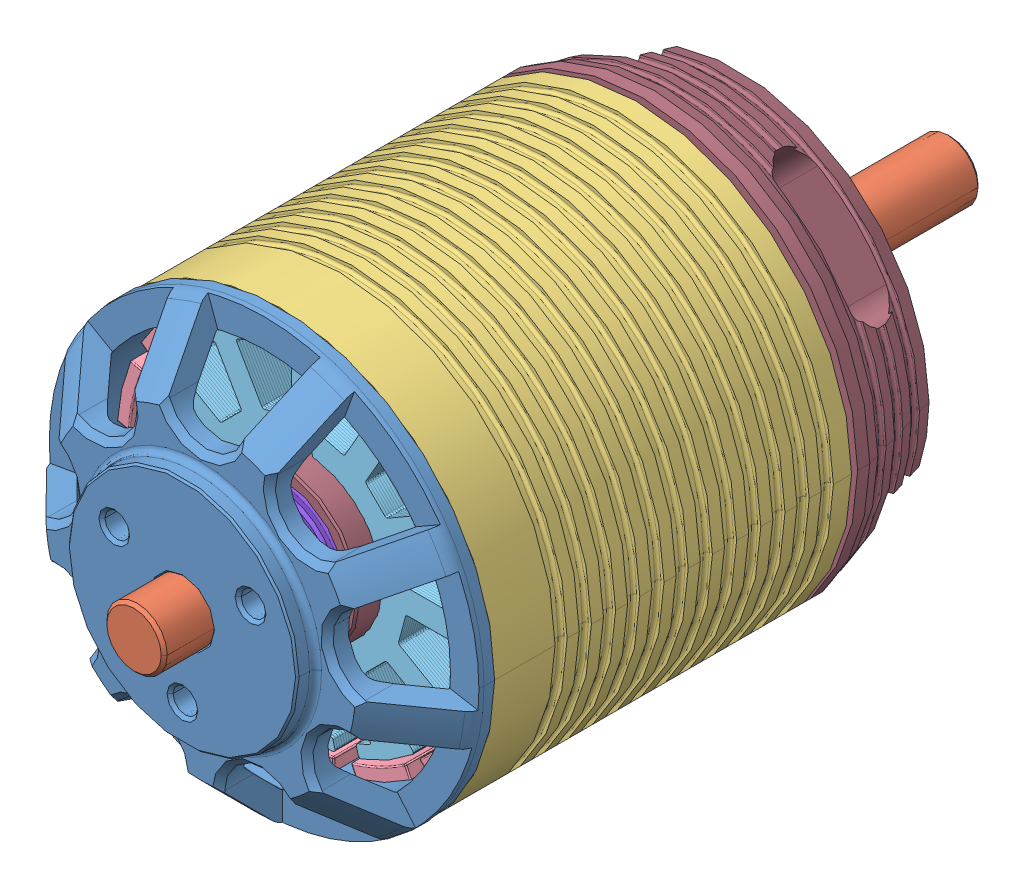
SolidWorks assembly BA-2826-Motor, configuration Default. Lengths in mm. (continued)
Components (placement in the parent): (continued)
- BA-2826-Motor(2)^BA-2826-Motor-1: BA-2826-Motor(2)^BA-2826-Motor [Default] at origin size (35.6 35.6 67.5) (virtual) (continued)
  - 2826-Stator-Mount^BA-2826-Motor(2)_BA-2826-Motor-1: 2826-Stator-Mount^BA-2826-Motor(2)_BA-2826-Motor [Default] at (-12.4646 -13.2477 18.5701) size (35.6 35.6 38.01) (virtual) (continued)
    - 28x13x26mm-Stator^2826-Stator-Mount_BA-2826-Motor(2)_BA-2826-Motor-1: 28x13x26mm-Stator^2826-Stator-Mount_BA-2826-Motor(2)_BA-2826-Motor [Default] at (-35.5349 -3.2376 -36.4185) size (28 28 26) (virtual) (continued)
      - 28x13x5mm-Stator^28x13x26mm-Stator_2826-Stator-Mount_BA-2826-Motor(2)_BA-2826-Motor-4: 28x13x5mm-Stator^28x13x26mm-Stator_2826-Stator-Mount_BA-2826-Motor(2)_BA-2826-Motor [Default] at (6.5198 12.3714 10.0893) size (28 28 5) (virtual)
        - 28x13x1mm-Stator^28x13x5mm-Stator_28x13x26mm-Stator_2826-Stator-Mount_BA-2826-Motor(2)_BA-2826-Motor-1: 28x13x1mm-Stator^28x13x5mm-Stator_28x13x26mm-Stator_2826-Stator-Mount_BA-2826-Motor(2)_BA-2826-Motor [Default] at (34.0086 1.4103 18.4307) size (28 28 1) (virtual)
          - 28x13-Stator Plate^28x13x1mm-Stator_28x13x5mm-Stator_28x13x26mm-Stator_2826-Stator-Mount_BA-2826-Motor(2)_BA-2826-Motor-1: 28x13-Stator Plate^28x13x1mm-Stator_28x13x5mm-Stator_28x13x26mm-Stator_2826-Stator-Mount_BA-2826-Motor(2)_BA-2826-Motor [Default] at (-28.2175 12.5042 6.2948) size (28 28 0.2) (virtual)
          - 28x13-Stator Plate^28x13x1mm-Stator_28x13x5mm-Stator_28x13x26mm-Stator_2826-Stator-Mount_BA-2826-Motor(2)_BA-2826-Motor-2: 28x13-Stator Plate^28x13x1mm-Stator_28x13x5mm-Stator_28x13x26mm-Stator_2826-Stator-Mount_BA-2826-Motor(2)_BA-2826-Motor [Default] at (-28.2175 12.5042 6.0948) size (28 28 0.2) (virtual)
          - 28x13-Stator Plate^28x13x1mm-Stator_28x13x5mm-Stator_28x13x26mm-Stator_2826-Stator-Mount_BA-2826-Motor(2)_BA-2826-Motor-3: 28x13-Stator Plate^28x13x1mm-Stator_28x13x5mm-Stator_28x13x26mm-Stator_2826-Stator-Mount_BA-2826-Motor(2)_BA-2826-Motor [Default] at (-28.2175 12.5042 5.8948) size (28 28 0.2) (virtual)
          - 28x13-Stator Plate^28x13x1mm-Stator_28x13x5mm-Stator_28x13x26mm-Stator_2826-Stator-Mount_BA-2826-Motor(2)_BA-2826-Motor-4: 28x13-Stator Plate^28x13x1mm-Stator_28x13x5mm-Stator_28x13x26mm-Stator_2826-Stator-Mount_BA-2826-Motor(2)_BA-2826-Motor [Default] at (-28.2175 12.5042 5.6948) size (28 28 0.2) (virtual)
          - 28x13-Stator Plate^28x13x1mm-Stator_28x13x5mm-Stator_28x13x26mm-Stator_2826-Stator-Mount_BA-2826-Motor(2)_BA-2826-Motor-5: 28x13-Stator Plate^28x13x1mm-Stator_28x13x5mm-Stator_28x13x26mm-Stator_2826-Stator-Mount_BA-2826-Motor(2)_BA-2826-Motor [Default] at (-28.2175 12.5042 5.4948) size (28 28 0.2) (virtual)
        - 28x13x1mm-Stator^28x13x5mm-Stator_28x13x26mm-Stator_2826-Stator-Mount_BA-2826-Motor(2)_BA-2826-Motor-2: 28x13x1mm-Stator^28x13x5mm-Stator_28x13x26mm-Stator_2826-Stator-Mount_BA-2826-Motor(2)_BA-2826-Motor [Default] at (34.0086 1.4103 17.4307) size (28 28 1) (virtual)
          - 28x13-Stator Plate^28x13x1mm-Stator_28x13x5mm-Stator_28x13x26mm-Stator_2826-Stator-Mount_BA-2826-Motor(2)_BA-2826-Motor-1: 28x13-Stator Plate^28x13x1mm-Stator_28x13x5mm-Stator_28x13x26mm-Stator_2826-Stator-Mount_BA-2826-Motor(2)_BA-2826-Motor [Default] at (-28.2175 12.5042 6.2948) size (28 28 0.2) (virtual)
          - 28x13-Stator Plate^28x13x1mm-Stator_28x13x5mm-Stator_28x13x26mm-Stator_2826-Stator-Mount_BA-2826-Motor(2)_BA-2826-Motor-2: 28x13-Stator Plate^28x13x1mm-Stator_28x13x5mm-Stator_28x13x26mm-Stator_2826-Stator-Mount_BA-2826-Motor(2)_BA-2826-Motor [Default] at (-28.2175 12.5042 6.0948) size (28 28 0.2) (virtual)
          - 28x13-Stator Plate^28x13x1mm-Stator_28x13x5mm-Stator_28x13x26mm-Stator_2826-Stator-Mount_BA-2826-Motor(2)_BA-2826-Motor-3: 28x13-Stator Plate^28x13x1mm-Stator_28x13x5mm-Stator_28x13x26mm-Stator_2826-Stator-Mount_BA-2826-Motor(2)_BA-2826-Motor [Default] at (-28.2175 12.5042 5.8948) size (28 28 0.2) (virtual)
          - 28x13-Stator Plate^28x13x1mm-Stator_28x13x5mm-Stator_28x13x26mm-Stator_2826-Stator-Mount_BA-2826-Motor(2)_BA-2826-Motor-4: 28x13-Stator Plate^28x13x1mm-Stator_28x13x5mm-Stator_28x13x26mm-Stator_2826-Stator-Mount_BA-2826-Motor(2)_BA-2826-Motor [Default] at (-28.2175 12.5042 5.6948) size (28 28 0.2) (virtual)
          - 28x13-Stator Plate^28x13x1mm-Stator_28x13x5mm-Stator_28x13x26mm-Stator_2826-Stator-Mount_BA-2826-Motor(2)_BA-2826-Motor-5: 28x13-Stator Plate^28x13x1mm-Stator_28x13x5mm-Stator_28x13x26mm-Stator_2826-Stator-Mount_BA-2826-Motor(2)_BA-2826-Motor [Default] at (-28.2175 12.5042 5.4948) size (28 28 0.2) (virtual)
        - 28x13x1mm-Stator^28x13x5mm-Stator_28x13x26mm-Stator_2826-Stator-Mount_BA-2826-Motor(2)_BA-2826-Motor-3: 28x13x1mm-Stator^28x13x5mm-Stator_28x13x26mm-Stator_2826-Stator-Mount_BA-2826-Motor(2)_BA-2826-Motor [Default] at (34.0086 1.4103 16.4307) size (28 28 1) (virtual)
          - 28x13-Stator Plate^28x13x1mm-Stator_28x13x5mm-Stator_28x13x26mm-Stator_2826-Stator-Mount_BA-2826-Motor(2)_BA-2826-Motor-1: 28x13-Stator Plate^28x13x1mm-Stator_28x13x5mm-Stator_28x13x26mm-Stator_2826-Stator-Mount_BA-2826-Motor(2)_BA-2826-Motor [Default] at (-28.2175 12.5042 6.2948) size (28 28 0.2) (virtual)
          - 28x13-Stator Plate^28x13x1mm-Stator_28x13x5mm-Stator_28x13x26mm-Stator_2826-Stator-Mount_BA-2826-Motor(2)_BA-2826-Motor-2: 28x13-Stator Plate^28x13x1mm-Stator_28x13x5mm-Stator_28x13x26mm-Stator_2826-Stator-Mount_BA-2826-Motor(2)_BA-2826-Motor [Default] at (-28.2175 12.5042 6.0948) size (28 28 0.2) (virtual)
          - 28x13-Stator Plate^28x13x1mm-Stator_28x13x5mm-Stator_28x13x26mm-Stator_2826-Stator-Mount_BA-2826-Motor(2)_BA-2826-Motor-3: 28x13-Stator Plate^28x13x1mm-Stator_28x13x5mm-Stator_28x13x26mm-Stator_2826-Stator-Mount_BA-2826-Motor(2)_BA-2826-Motor [Default] at (-28.2175 12.5042 5.8948) size (28 28 0.2) (virtual)
          - 28x13-Stator Plate^28x13x1mm-Stator_28x13x5mm-Stator_28x13x26mm-Stator_2826-Stator-Mount_BA-2826-Motor(2)_BA-2826-Motor-4: 28x13-Stator Plate^28x13x1mm-Stator_28x13x5mm-Stator_28x13x26mm-Stator_2826-Stator-Mount_BA-2826-Motor(2)_BA-2826-Motor [Default] at (-28.2175 12.5042 5.6948) size (28 28 0.2) (virtual)
          - 28x13-Stator Plate^28x13x1mm-Stator_28x13x5mm-Stator_28x13x26mm-Stator_2826-Stator-Mount_BA-2826-Motor(2)_BA-2826-Motor-5: 28x13-Stator Plate^28x13x1mm-Stator_28x13x5mm-Stator_28x13x26mm-Stator_2826-Stator-Mount_BA-2826-Motor(2)_BA-2826-Motor [Default] at (-28.2175 12.5042 5.4948) size (28 28 0.2) (virtual)
        - 28x13x1mm-Stator^28x13x5mm-Stator_28x13x26mm-Stator_2826-Stator-Mount_BA-2826-Motor(2)_BA-2826-Motor-4: 28x13x1mm-Stator^28x13x5mm-Stator_28x13x26mm-Stator_2826-Stator-Mount_BA-2826-Motor(2)_BA-2826-Motor [Default] at (34.0086 1.4103 15.4307) size (28 28 1) (virtual)
          - 28x13-Stator Plate^28x13x1mm-Stator_28x13x5mm-Stator_28x13x26mm-Stator_2826-Stator-Mount_BA-2826-Motor(2)_BA-2826-Motor-1: 28x13-Stator Plate^28x13x1mm-Stator_28x13x5mm-Stator_28x13x26mm-Stator_2826-Stator-Mount_BA-2826-Motor(2)_BA-2826-Motor [Default] at (-28.2175 12.5042 6.2948) size (28 28 0.2) (virtual)
          - 28x13-Stator Plate^28x13x1mm-Stator_28x13x5mm-Stator_28x13x26mm-Stator_2826-Stator-Mount_BA-2826-Motor(2)_BA-2826-Motor-2: 28x13-Stator Plate^28x13x1mm-Stator_28x13x5mm-Stator_28x13x26mm-Stator_2826-Stator-Mount_BA-2826-Motor(2)_BA-2826-Motor [Default] at (-28.2175 12.5042 6.0948) size (28 28 0.2) (virtual)
          - 28x13-Stator Plate^28x13x1mm-Stator_28x13x5mm-Stator_28x13x26mm-Stator_2826-Stator-Mount_BA-2826-Motor(2)_BA-2826-Motor-3: 28x13-Stator Plate^28x13x1mm-Stator_28x13x5mm-Stator_28x13x26mm-Stator_2826-Stator-Mount_BA-2826-Motor(2)_BA-2826-Motor [Default] at (-28.2175 12.5042 5.8948) size (28 28 0.2) (virtual)
          - 28x13-Stator Plate^28x13x1mm-Stator_28x13x5mm-Stator_28x13x26mm-Stator_2826-Stator-Mount_BA-2826-Motor(2)_BA-2826-Motor-4: 28x13-Stator Plate^28x13x1mm-Stator_28x13x5mm-Stator_28x13x26mm-Stator_2826-Stator-Mount_BA-2826-Motor(2)_BA-2826-Motor [Default] at (-28.2175 12.5042 5.6948) size (28 28 0.2) (virtual)
          - 28x13-Stator Plate^28x13x1mm-Stator_28x13x5mm-Stator_28x13x26mm-Stator_2826-Stator-Mount_BA-2826-Motor(2)_BA-2826-Motor-5: 28x13-Stator Plate^28x13x1mm-Stator_28x13x5mm-Stator_28x13x26mm-Stator_2826-Stator-Mount_BA-2826-Motor(2)_BA-2826-Motor [Default] at (-28.2175 12.5042 5.4948) size (28 28 0.2) (virtual)
        - 28x13x1mm-Stator^28x13x5mm-Stator_28x13x26mm-Stator_2826-Stator-Mount_BA-2826-Motor(2)_BA-2826-Motor-5: 28x13x1mm-Stator^28x13x5mm-Stator_28x13x26mm-Stator_2826-Stator-Mount_BA-2826-Motor(2)_BA-2826-Motor [Default] at (34.0086 1.4103 14.4307) size (28 28 1) (virtual)
          - 28x13-Stator Plate^28x13x1mm-Stator_28x13x5mm-Stator_28x13x26mm-Stator_2826-Stator-Mount_BA-2826-Motor(2)_BA-2826-Motor-1: 28x13-Stator Plate^28x13x1mm-Stator_28x13x5mm-Stator_28x13x26mm-Stator_2826-Stator-Mount_BA-2826-Motor(2)_BA-2826-Motor [Default] at (-28.2175 12.5042 6.2948) size (28 28 0.2) (virtual)
          - 28x13-Stator Plate^28x13x1mm-Stator_28x13x5mm-Stator_28x13x26mm-Stator_2826-Stator-Mount_BA-2826-Motor(2)_BA-2826-Motor-2: 28x13-Stator Plate^28x13x1mm-Stator_28x13x5mm-Stator_28x13x26mm-Stator_2826-Stator-Mount_BA-2826-Motor(2)_BA-2826-Motor [Default] at (-28.2175 12.5042 6.0948) size (28 28 0.2) (virtual)
          - 28x13-Stator Plate^28x13x1mm-Stator_28x13x5mm-Stator_28x13x26mm-Stator_2826-Stator-Mount_BA-2826-Motor(2)_BA-2826-Motor-3: 28x13-Stator Plate^28x13x1mm-Stator_28x13x5mm-Stator_28x13x26mm-Stator_2826-Stator-Mount_BA-2826-Motor(2)_BA-2826-Motor [Default] at (-28.2175 12.5042 5.8948) size (28 28 0.2) (virtual)
          - 28x13-Stator Plate^28x13x1mm-Stator_28x13x5mm-Stator_28x13x26mm-Stator_2826-Stator-Mount_BA-2826-Motor(2)_BA-2826-Motor-4: 28x13-Stator Plate^28x13x1mm-Stator_28x13x5mm-Stator_28x13x26mm-Stator_2826-Stator-Mount_BA-2826-Motor(2)_BA-2826-Motor [Default] at (-28.2175 12.5042 5.6948) size (28 28 0.2) (virtual)
          - 28x13-Stator Plate^28x13x1mm-Stator_28x13x5mm-Stator_28x13x26mm-Stator_2826-Stator-Mount_BA-2826-Motor(2)_BA-2826-Motor-5: 28x13-Stator Plate^28x13x1mm-Stator_28x13x5mm-Stator_28x13x26mm-Stator_2826-Stator-Mount_BA-2826-Motor(2)_BA-2826-Motor [Default] at (-28.2175 12.5042 5.4948) size (28 28 0.2) (virtual)
      - 28x13x5mm-Stator^28x13x26mm-Stator_2826-Stator-Mount_BA-2826-Motor(2)_BA-2826-Motor-5: 28x13x5mm-Stator^28x13x26mm-Stator_2826-Stator-Mount_BA-2826-Motor(2)_BA-2826-Motor [Default] at (6.5198 12.3714 5.0893) size (28 28 5) (virtual)
        - 28x13x1mm-Stator^28x13x5mm-Stator_28x13x26mm-Stator_2826-Stator-Mount_BA-2826-Motor(2)_BA-2826-Motor-1: 28x13x1mm-Stator^28x13x5mm-Stator_28x13x26mm-Stator_2826-Stator-Mount_BA-2826-Motor(2)_BA-2826-Motor [Default] at (34.0086 1.4103 18.4307) size (28 28 1) (virtual)
          - 28x13-Stator Plate^28x13x1mm-Stator_28x13x5mm-Stator_28x13x26mm-Stator_2826-Stator-Mount_BA-2826-Motor(2)_BA-2826-Motor-1: 28x13-Stator Plate^28x13x1mm-Stator_28x13x5mm-Stator_28x13x26mm-Stator_2826-Stator-Mount_BA-2826-Motor(2)_BA-2826-Motor [Default] at (-28.2175 12.5042 6.2948) size (28 28 0.2) (virtual)
          - 28x13-Stator Plate^28x13x1mm-Stator_28x13x5mm-Stator_28x13x26mm-Stator_2826-Stator-Mount_BA-2826-Motor(2)_BA-2826-Motor-2: 28x13-Stator Plate^28x13x1mm-Stator_28x13x5mm-Stator_28x13x26mm-Stator_2826-Stator-Mount_BA-2826-Motor(2)_BA-2826-Motor [Default] at (-28.2175 12.5042 6.0948) size (28 28 0.2) (virtual)
          - 28x13-Stator Plate^28x13x1mm-Stator_28x13x5mm-Stator_28x13x26mm-Stator_2826-Stator-Mount_BA-2826-Motor(2)_BA-2826-Motor-3: 28x13-Stator Plate^28x13x1mm-Stator_28x13x5mm-Stator_28x13x26mm-Stator_2826-Stator-Mount_BA-2826-Motor(2)_BA-2826-Motor [Default] at (-28.2175 12.5042 5.8948) size (28 28 0.2) (virtual)
          - 28x13-Stator Plate^28x13x1mm-Stator_28x13x5mm-Stator_28x13x26mm-Stator_2826-Stator-Mount_BA-2826-Motor(2)_BA-2826-Motor-4: 28x13-Stator Plate^28x13x1mm-Stator_28x13x5mm-Stator_28x13x26mm-Stator_2826-Stator-Mount_BA-2826-Motor(2)_BA-2826-Motor [Default] at (-28.2175 12.5042 5.6948) size (28 28 0.2) (virtual)
          - 28x13-Stator Plate^28x13x1mm-Stator_28x13x5mm-Stator_28x13x26mm-Stator_2826-Stator-Mount_BA-2826-Motor(2)_BA-2826-Motor-5: 28x13-Stator Plate^28x13x1mm-Stator_28x13x5mm-Stator_28x13x26mm-Stator_2826-Stator-Mount_BA-2826-Motor(2)_BA-2826-Motor [Default] at (-28.2175 12.5042 5.4948) size (28 28 0.2) (virtual)
        - 28x13x1mm-Stator^28x13x5mm-Stator_28x13x26mm-Stator_2826-Stator-Mount_BA-2826-Motor(2)_BA-2826-Motor-2: 28x13x1mm-Stator^28x13x5mm-Stator_28x13x26mm-Stator_2826-Stator-Mount_BA-2826-Motor(2)_BA-2826-Motor [Default] at (34.0086 1.4103 17.4307) size (28 28 1) (virtual)
          - 28x13-Stator Plate^28x13x1mm-Stator_28x13x5mm-Stator_28x13x26mm-Stator_2826-Stator-Mount_BA-2826-Motor(2)_BA-2826-Motor-1: 28x13-Stator Plate^28x13x1mm-Stator_28x13x5mm-Stator_28x13x26mm-Stator_2826-Stator-Mount_BA-2826-Motor(2)_BA-2826-Motor [Default] at (-28.2175 12.5042 6.2948) size (28 28 0.2) (virtual)
          - 28x13-Stator Plate^28x13x1mm-Stator_28x13x5mm-Stator_28x13x26mm-Stator_2826-Stator-Mount_BA-2826-Motor(2)_BA-2826-Motor-2: 28x13-Stator Plate^28x13x1mm-Stator_28x13x5mm-Stator_28x13x26mm-Stator_2826-Stator-Mount_BA-2826-Motor(2)_BA-2826-Motor [Default] at (-28.2175 12.5042 6.0948) size (28 28 0.2) (virtual)
          - 28x13-Stator Plate^28x13x1mm-Stator_28x13x5mm-Stator_28x13x26mm-Stator_2826-Stator-Mount_BA-2826-Motor(2)_BA-2826-Motor-3: 28x13-Stator Plate^28x13x1mm-Stator_28x13x5mm-Stator_28x13x26mm-Stator_2826-Stator-Mount_BA-2826-Motor(2)_BA-2826-Motor [Default] at (-28.2175 12.5042 5.8948) size (28 28 0.2) (virtual)
          - 28x13-Stator Plate^28x13x1mm-Stator_28x13x5mm-Stator_28x13x26mm-Stator_2826-Stator-Mount_BA-2826-Motor(2)_BA-2826-Motor-4: 28x13-Stator Plate^28x13x1mm-Stator_28x13x5mm-Stator_28x13x26mm-Stator_2826-Stator-Mount_BA-2826-Motor(2)_BA-2826-Motor [Default] at (-28.2175 12.5042 5.6948) size (28 28 0.2) (virtual)
          - 28x13-Stator Plate^28x13x1mm-Stator_28x13x5mm-Stator_28x13x26mm-Stator_2826-Stator-Mount_BA-2826-Motor(2)_BA-2826-Motor-5: 28x13-Stator Plate^28x13x1mm-Stator_28x13x5mm-Stator_28x13x26mm-Stator_2826-Stator-Mount_BA-2826-Motor(2)_BA-2826-Motor [Default] at (-28.2175 12.5042 5.4948) size (28 28 0.2) (virtual)
        - 28x13x1mm-Stator^28x13x5mm-Stator_28x13x26mm-Stator_2826-Stator-Mount_BA-2826-Motor(2)_BA-2826-Motor-3: 28x13x1mm-Stator^28x13x5mm-Stator_28x13x26mm-Stator_2826-Stator-Mount_BA-2826-Motor(2)_BA-2826-Motor [Default] at (34.0086 1.4103 16.4307) size (28 28 1) (virtual)
          - 28x13-Stator Plate^28x13x1mm-Stator_28x13x5mm-Stator_28x13x26mm-Stator_2826-Stator-Mount_BA-2826-Motor(2)_BA-2826-Motor-1: 28x13-Stator Plate^28x13x1mm-Stator_28x13x5mm-Stator_28x13x26mm-Stator_2826-Stator-Mount_BA-2826-Motor(2)_BA-2826-Motor [Default] at (-28.2175 12.5042 6.2948) size (28 28 0.2) (virtual)
          - 28x13-Stator Plate^28x13x1mm-Stator_28x13x5mm-Stator_28x13x26mm-Stator_2826-Stator-Mount_BA-2826-Motor(2)_BA-2826-Motor-2: 28x13-Stator Plate^28x13x1mm-Stator_28x13x5mm-Stator_28x13x26mm-Stator_2826-Stator-Mount_BA-2826-Motor(2)_BA-2826-Motor [Default] at (-28.2175 12.5042 6.0948) size (28 28 0.2) (virtual)
          - 28x13-Stator Plate^28x13x1mm-Stator_28x13x5mm-Stator_28x13x26mm-Stator_2826-Stator-Mount_BA-2826-Motor(2)_BA-2826-Motor-3: 28x13-Stator Plate^28x13x1mm-Stator_28x13x5mm-Stator_28x13x26mm-Stator_2826-Stator-Mount_BA-2826-Motor(2)_BA-2826-Motor [Default] at (-28.2175 12.5042 5.8948) size (28 28 0.2) (virtual)
          - 28x13-Stator Plate^28x13x1mm-Stator_28x13x5mm-Stator_28x13x26mm-Stator_2826-Stator-Mount_BA-2826-Motor(2)_BA-2826-Motor-4: 28x13-Stator Plate^28x13x1mm-Stator_28x13x5mm-Stator_28x13x26mm-Stator_2826-Stator-Mount_BA-2826-Motor(2)_BA-2826-Motor [Default] at (-28.2175 12.5042 5.6948) size (28 28 0.2) (virtual)
          - 28x13-Stator Plate^28x13x1mm-Stator_28x13x5mm-Stator_28x13x26mm-Stator_2826-Stator-Mount_BA-2826-Motor(2)_BA-2826-Motor-5: 28x13-Stator Plate^28x13x1mm-Stator_28x13x5mm-Stator_28x13x26mm-Stator_2826-Stator-Mount_BA-2826-Motor(2)_BA-2826-Motor [Default] at (-28.2175 12.5042 5.4948) size (28 28 0.2) (virtual)
        - 28x13x1mm-Stator^28x13x5mm-Stator_28x13x26mm-Stator_2826-Stator-Mount_BA-2826-Motor(2)_BA-2826-Motor-4: 28x13x1mm-Stator^28x13x5mm-Stator_28x13x26mm-Stator_2826-Stator-Mount_BA-2826-Motor(2)_BA-2826-Motor [Default] at (34.0086 1.4103 15.4307) size (28 28 1) (virtual)
          - 28x13-Stator Plate^28x13x1mm-Stator_28x13x5mm-Stator_28x13x26mm-Stator_2826-Stator-Mount_BA-2826-Motor(2)_BA-2826-Motor-1: 28x13-Stator Plate^28x13x1mm-Stator_28x13x5mm-Stator_28x13x26mm-Stator_2826-Stator-Mount_BA-2826-Motor(2)_BA-2826-Motor [Default] at (-28.2175 12.5042 6.2948) size (28 28 0.2) (virtual)
          - 28x13-Stator Plate^28x13x1mm-Stator_28x13x5mm-Stator_28x13x26mm-Stator_2826-Stator-Mount_BA-2826-Motor(2)_BA-2826-Motor-2: 28x13-Stator Plate^28x13x1mm-Stator_28x13x5mm-Stator_28x13x26mm-Stator_2826-Stator-Mount_BA-2826-Motor(2)_BA-2826-Motor [Default] at (-28.2175 12.5042 6.0948) size (28 28 0.2) (virtual)
          - 28x13-Stator Plate^28x13x1mm-Stator_28x13x5mm-Stator_28x13x26mm-Stator_2826-Stator-Mount_BA-2826-Motor(2)_BA-2826-Motor-3: 28x13-Stator Plate^28x13x1mm-Stator_28x13x5mm-Stator_28x13x26mm-Stator_2826-Stator-Mount_BA-2826-Motor(2)_BA-2826-Motor [Default] at (-28.2175 12.5042 5.8948) size (28 28 0.2) (virtual)
          - 28x13-Stator Plate^28x13x1mm-Stator_28x13x5mm-Stator_28x13x26mm-Stator_2826-Stator-Mount_BA-2826-Motor(2)_BA-2826-Motor-4: 28x13-Stator Plate^28x13x1mm-Stator_28x13x5mm-Stator_28x13x26mm-Stator_2826-Stator-Mount_BA-2826-Motor(2)_BA-2826-Motor [Default] at (-28.2175 12.5042 5.6948) size (28 28 0.2) (virtual)
          - 28x13-Stator Plate^28x13x1mm-Stator_28x13x5mm-Stator_28x13x26mm-Stator_2826-Stator-Mount_BA-2826-Motor(2)_BA-2826-Motor-5: 28x13-Stator Plate^28x13x1mm-Stator_28x13x5mm-Stator_28x13x26mm-Stator_2826-Stator-Mount_BA-2826-Motor(2)_BA-2826-Motor [Default] at (-28.2175 12.5042 5.4948) size (28 28 0.2) (virtual)
        - 28x13x1mm-Stator^28x13x5mm-Stator_28x13x26mm-Stator_2826-Stator-Mount_BA-2826-Motor(2)_BA-2826-Motor-5: 28x13x1mm-Stator^28x13x5mm-Stator_28x13x26mm-Stator_2826-Stator-Mount_BA-2826-Motor(2)_BA-2826-Motor [Default] at (34.0086 1.4103 14.4307) size (28 28 1) (virtual)
          - 28x13-Stator Plate^28x13x1mm-Stator_28x13x5mm-Stator_28x13x26mm-Stator_2826-Stator-Mount_BA-2826-Motor(2)_BA-2826-Motor-1: 28x13-Stator Plate^28x13x1mm-Stator_28x13x5mm-Stator_28x13x26mm-Stator_2826-Stator-Mount_BA-2826-Motor(2)_BA-2826-Motor [Default] at (-28.2175 12.5042 6.2948) size (28 28 0.2) (virtual)
          - 28x13-Stator Plate^28x13x1mm-Stator_28x13x5mm-Stator_28x13x26mm-Stator_2826-Stator-Mount_BA-2826-Motor(2)_BA-2826-Motor-2: 28x13-Stator Plate^28x13x1mm-Stator_28x13x5mm-Stator_28x13x26mm-Stator_2826-Stator-Mount_BA-2826-Motor(2)_BA-2826-Motor [Default] at (-28.2175 12.5042 6.0948) size (28 28 0.2) (virtual)
          - 28x13-Stator Plate^28x13x1mm-Stator_28x13x5mm-Stator_28x13x26mm-Stator_2826-Stator-Mount_BA-2826-Motor(2)_BA-2826-Motor-3: 28x13-Stator Plate^28x13x1mm-Stator_28x13x5mm-Stator_28x13x26mm-Stator_2826-Stator-Mount_BA-2826-Motor(2)_BA-2826-Motor [Default] at (-28.2175 12.5042 5.8948) size (28 28 0.2) (virtual)
          - 28x13-Stator Plate^28x13x1mm-Stator_28x13x5mm-Stator_28x13x26mm-Stator_2826-Stator-Mount_BA-2826-Motor(2)_BA-2826-Motor-4: 28x13-Stator Plate^28x13x1mm-Stator_28x13x5mm-Stator_28x13x26mm-Stator_2826-Stator-Mount_BA-2826-Motor(2)_BA-2826-Motor [Default] at (-28.2175 12.5042 5.6948) size (28 28 0.2) (virtual)
          - 28x13-Stator Plate^28x13x1mm-Stator_28x13x5mm-Stator_28x13x26mm-Stator_2826-Stator-Mount_BA-2826-Motor(2)_BA-2826-Motor-5: 28x13-Stator Plate^28x13x1mm-Stator_28x13x5mm-Stator_28x13x26mm-Stator_2826-Stator-Mount_BA-2826-Motor(2)_BA-2826-Motor [Default] at (-28.2175 12.5042 5.4948) size (28 28 0.2) (virtual)
      - 28x13x1mm-Stator^28x13x26mm-Stator_2826-Stator-Mount_BA-2826-Motor(2)_BA-2826-Motor-1: 28x13x1mm-Stator^28x13x26mm-Stator_2826-Stator-Mount_BA-2826-Motor(2)_BA-2826-Motor [Default] at (40.5284 13.7817 18.52) size (28 28 1) (virtual)
        - 28x13-Stator Plate^28x13x1mm-Stator_28x13x26mm-Stator_2826-Stator-Mount_BA-2826-Motor(2)_BA-2826-Motor-1: 28x13-Stator Plate^28x13x1mm-Stator_28x13x26mm-Stator_2826-Stator-Mount_BA-2826-Motor(2)_BA-2826-Motor [Default] at (-28.2175 12.5042 6.2948) size (28 28 0.2) (virtual)
        - 28x13-Stator Plate^28x13x1mm-Stator_28x13x26mm-Stator_2826-Stator-Mount_BA-2826-Motor(2)_BA-2826-Motor-2: 28x13-Stator Plate^28x13x1mm-Stator_28x13x26mm-Stator_2826-Stator-Mount_BA-2826-Motor(2)_BA-2826-Motor [Default] at (-28.2175 12.5042 6.0948) size (28 28 0.2) (virtual)
        - 28x13-Stator Plate^28x13x1mm-Stator_28x13x26mm-Stator_2826-Stator-Mount_BA-2826-Motor(2)_BA-2826-Motor-3: 28x13-Stator Plate^28x13x1mm-Stator_28x13x26mm-Stator_2826-Stator-Mount_BA-2826-Motor(2)_BA-2826-Motor [Default] at (-28.2175 12.5042 5.8948) size (28 28 0.2) (virtual)
        - 28x13-Stator Plate^28x13x1mm-Stator_28x13x26mm-Stator_2826-Stator-Mount_BA-2826-Motor(2)_BA-2826-Motor-4: 28x13-Stator Plate^28x13x1mm-Stator_28x13x26mm-Stator_2826-Stator-Mount_BA-2826-Motor(2)_BA-2826-Motor [Default] at (-28.2175 12.5042 5.6948) size (28 28 0.2) (virtual)
        - 28x13-Stator Plate^28x13x1mm-Stator_28x13x26mm-Stator_2826-Stator-Mount_BA-2826-Motor(2)_BA-2826-Motor-5: 28x13-Stator Plate^28x13x1mm-Stator_28x13x26mm-Stator_2826-Stator-Mount_BA-2826-Motor(2)_BA-2826-Motor [Default] at (-28.2175 12.5042 5.4948) size (28 28 0.2) (virtual)
    - 5x11x5_Bearing_685HZZ^2826-Stator-Mount_BA-2826-Motor(2)_BA-2826-Motor-1: 5x11x5_Bearing_685HZZ^2826-Stator-Mount_BA-2826-Motor(2)_BA-2826-Motor [Default] at (-23.224 23.0483 8.0982) x (0 0 -1) z (0.999998 0.001828 0) size (5 11 11) (virtual)
      - 685HZZ_SOLID_1^5x11x5_Bearing_685HZZ_2826-Stator-Mount_BA-2826-Motor(2)_BA-2826-Motor-1: 685HZZ_SOLID_1^5x11x5_Bearing_685HZZ_2826-Stator-Mount_BA-2826-Motor(2)_BA-2826-Motor [Default] at origin size (5 6.35 6.35) (virtual)
      - 685HZZ_SOLID_2^5x11x5_Bearing_685HZZ_2826-Stator-Mount_BA-2826-Motor(2)_BA-2826-Motor-1: 685HZZ_SOLID_2^5x11x5_Bearing_685HZZ_2826-Stator-Mount_BA-2826-Motor(2)_BA-2826-Motor [Default] at origin size (5 11 11) (virtual)
      - 685HZZ_SOLID_3^5x11x5_Bearing_685HZZ_2826-Stator-Mount_BA-2826-Motor(2)_BA-2826-Motor-1: 685HZZ_SOLID_3^5x11x5_Bearing_685HZZ_2826-Stator-Mount_BA-2826-Motor(2)_BA-2826-Motor [Default] at origin size (2.94 9.96 10.15) (virtual)
    - 5x11x5_Bearing_685HZZ^2826-Stator-Mount_BA-2826-Motor(2)_BA-2826-Motor-2: 5x11x5_Bearing_685HZZ^2826-Stator-Mount_BA-2826-Motor(2)_BA-2826-Motor [Default] at (-23.224 23.0483 13.102) x (0 0 -1) z (0.999826 0.018655 0) size (5 11 11) (virtual)
      - 685HZZ_SOLID_1^5x11x5_Bearing_685HZZ_2826-Stator-Mount_BA-2826-Motor(2)_BA-2826-Motor-1: 685HZZ_SOLID_1^5x11x5_Bearing_685HZZ_2826-Stator-Mount_BA-2826-Motor(2)_BA-2826-Motor [Default] at origin size (5 6.35 6.35) (virtual)
      - 685HZZ_SOLID_2^5x11x5_Bearing_685HZZ_2826-Stator-Mount_BA-2826-Motor(2)_BA-2826-Motor-1: 685HZZ_SOLID_2^5x11x5_Bearing_685HZZ_2826-Stator-Mount_BA-2826-Motor(2)_BA-2826-Motor [Default] at origin size (5 11 11) (virtual)
      - 685HZZ_SOLID_3^5x11x5_Bearing_685HZZ_2826-Stator-Mount_BA-2826-Motor(2)_BA-2826-Motor-1: 685HZZ_SOLID_3^5x11x5_Bearing_685HZZ_2826-Stator-Mount_BA-2826-Motor(2)_BA-2826-Motor [Default] at origin size (2.94 9.96 10.15) (virtual)
    - 5x16x5_Bearing_625HZZ^2826-Stator-Mount_BA-2826-Motor(2)_BA-2826-Motor-1: 5x16x5_Bearing_625HZZ^2826-Stator-Mount_BA-2826-Motor(2)_BA-2826-Motor [Default] at (-23.224 23.0483 -19.4056) x (0 0 1) z (-0.998783 -0.049323 0) size (5 16 16) (virtual)
      - 625HZZ_SOLID_1^5x16x5_Bearing_625HZZ_2826-Stator-Mount_BA-2826-Motor(2)_BA-2826-Motor-1: 625HZZ_SOLID_1^5x16x5_Bearing_625HZZ_2826-Stator-Mount_BA-2826-Motor(2)_BA-2826-Motor [Default] at origin size (5 8.86 8.86) (virtual)
      - 625HZZ_SOLID_2^5x16x5_Bearing_625HZZ_2826-Stator-Mount_BA-2826-Motor(2)_BA-2826-Motor-1: 625HZZ_SOLID_2^5x16x5_Bearing_625HZZ_2826-Stator-Mount_BA-2826-Motor(2)_BA-2826-Motor [Default] at origin size (5 16 16) (virtual)
      - 625HZZ_SOLID_3^5x16x5_Bearing_625HZZ_2826-Stator-Mount_BA-2826-Motor(2)_BA-2826-Motor-1: 625HZZ_SOLID_3^5x16x5_Bearing_625HZZ_2826-Stator-Mount_BA-2826-Motor(2)_BA-2826-Motor [Default] at origin size (2.94 12.54 12.7) (virtual)
    - 2826-Mount^2826-Stator-Mount_BA-2826-Motor(2)_BA-2826-Motor-1: 2826-Mount^2826-Stator-Mount_BA-2826-Motor(2)_BA-2826-Motor [Default] at (-23.224 23.0483 -22.4037) size (35.6 35.6 38) (virtual)
  - Spacer-5mm(2)^BA-2826-Motor(2)_BA-2826-Motor-1: Spacer-5mm(2)^BA-2826-Motor(2)_BA-2826-Motor [Default] at (-35.6886 9.8006 34.174) size (7 7 0.5) (virtual)
  - Spacer-5mm(2)^BA-2826-Motor(2)_BA-2826-Motor-2: Spacer-5mm(2)^BA-2826-Motor(2)_BA-2826-Motor [Default] at (-35.6886 9.8006 -3.8374) size (7 7 0.5) (virtual)
  - Collar-5mm(2)^BA-2826-Motor(2)_BA-2826-Motor-1: Collar-5mm(2)^BA-2826-Motor(2)_BA-2826-Motor [Default] at (-35.6886 9.8006 -8.8374) x (0.013364 0.999911 0) z (0 0 1) size (11 11 5) (virtual)
